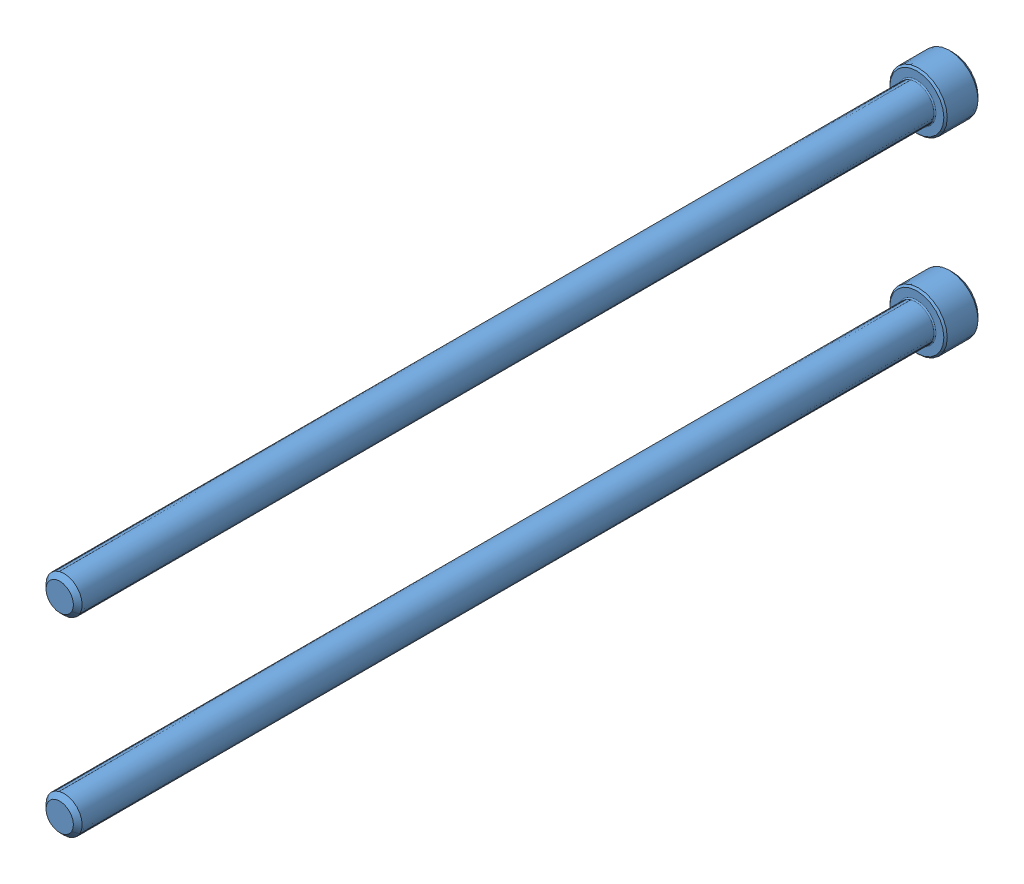
SolidWorks assembly WCP - GreyT Elevator (Cascade, 2 Stage) (1).step, configuration Default. Lengths in mm. (continued)
Components (placement in the parent): (continued)
- 10-32 SHCS - No Thread_WCP-0274 - 4.500.step-2: 10-32 SHCS - No Thread_WCP-0274 - 4.500.step [Default] at (165.1 1193.8 -77.7875) x (0.495006 -0.86889 0) z (0.86889 0.495006 0) size (7.67 119.13 7.67) (hidden)
- WCP-0326 Rev1.step-1: WCP-0326 Rev1.step [Default] at (165.1 1168.4 27.7749) x (0.127192 0.991878 0) z (0.991878 -0.127192 0) size (11.02 4.76 11) (hidden)
- WCP-0326 Rev1.step-2: WCP-0326 Rev1.step [Default] at (165.1 1193.8 27.7749) x (0.127192 0.991878 0) z (0.991878 -0.127192 0) size (11.02 4.76 11) (hidden)
- 10-32 BHCS - No Thread_WCP-0257 - 1.500.step-1: 10-32 BHCS - No Thread_WCP-0257 - 1.500.step [Default] at (101.6 1168.4 -101.6) x (-0.802481 0.596678 0) z (-0.596678 -0.802481 0) size (9.17 40.67 9.17) (hidden)
- 10-32 BHCS - No Thread_WCP-0257 - 1.500.step-2: 10-32 BHCS - No Thread_WCP-0257 - 1.500.step [Default] at (101.6 1193.8 -101.6) x (-0.802481 0.596678 0) z (-0.596678 -0.802481 0) size (9.17 40.67 9.17) (hidden)
- 10-32 BHCS - No Thread_WCP-0257 - 1.500.step-3: 10-32 BHCS - No Thread_WCP-0257 - 1.500.step [Default] at (76.2 1193.8 -101.6) x (-0.802481 0.596678 0) z (-0.596678 -0.802481 0) size (9.17 40.67 9.17) (hidden)
- 10-32 BHCS - No Thread_WCP-0257 - 1.500.step-4: 10-32 BHCS - No Thread_WCP-0257 - 1.500.step [Default] at (76.2 1168.4 -101.6) x (-0.802481 0.596678 0) z (-0.596678 -0.802481 0) size (9.17 40.67 9.17) (hidden)
- WCP-0326 Rev1.step-3: WCP-0326 Rev1.step [Default] at (101.6 1168.4 -67.4751) x (0.127192 0.991878 0) z (0.991878 -0.127192 0) size (11.02 4.76 11) (hidden)
- WCP-0326 Rev1.step-4: WCP-0326 Rev1.step [Default] at (101.6 1193.8 -67.4751) x (0.127192 0.991878 0) z (0.991878 -0.127192 0) size (11.02 4.76 11) (hidden)
- WCP-0326 Rev1.step-5: WCP-0326 Rev1.step [Default] at (76.2 1193.8 -67.4751) x (0.127192 0.991878 0) z (0.991878 -0.127192 0) size (11.02 4.76 11) (hidden)
- WCP-0326 Rev1.step-6: WCP-0326 Rev1.step [Default] at (76.2 1168.4 -67.4751) x (0.127192 0.991878 0) z (0.991878 -0.127192 0) size (11.02 4.76 11) (hidden)
- 10-32 BHCS - No Thread_WCP-0252 - 0.375.step-1: 10-32 BHCS - No Thread_WCP-0252 - 0.375.step [Default] at (165.1 11.1125 12.7) x (0.583861 0 0.811854) z (0.811854 0 -0.583861) size (9.17 12.1 9.17) (hidden)
- 10-32 BHCS - No Thread_WCP-0252 - 0.375.step-2: 10-32 BHCS - No Thread_WCP-0252 - 0.375.step [Default] at (165.1 11.1125 0) x (0.583861 0 0.811854) z (0.811854 0 -0.583861) size (9.17 12.1 9.17) (hidden)
- 10-32 BHCS - No Thread_WCP-0252 - 0.375.step-3: 10-32 BHCS - No Thread_WCP-0252 - 0.375.step [Default] at (165.1 11.1125 -12.7) x (0.583861 0 0.811854) z (0.811854 0 -0.583861) size (9.17 12.1 9.17) (hidden)
- 10-32 BHCS - No Thread_WCP-0252 - 0.375.step-4: 10-32 BHCS - No Thread_WCP-0252 - 0.375.step [Default] at (177.8 25.4 12.7) x (0 -0.948064 0.318079) z (0 0.318079 0.948064) size (9.17 12.1 9.17) (hidden)
- 10-32 BHCS - No Thread_WCP-0252 - 0.375.step-5: 10-32 BHCS - No Thread_WCP-0252 - 0.375.step [Default] at (177.8 25.4 0) x (0 -0.948064 0.318079) z (0 0.318079 0.948064) size (9.17 12.1 9.17) (hidden)
- 10-32 BHCS - No Thread_WCP-0252 - 0.375.step-6: 10-32 BHCS - No Thread_WCP-0252 - 0.375.step [Default] at (177.8 25.4 -12.7) x (0 -0.948064 0.318079) z (0 0.318079 0.948064) size (9.17 12.1 9.17) (hidden)
- 10-32 BHCS - No Thread_WCP-0252 - 0.375.step-7: 10-32 BHCS - No Thread_WCP-0252 - 0.375.step [Default] at (152.4 25.4 12.7) x (0 -0.983057 -0.183299) z (0 0.183299 -0.983057) size (9.17 12.1 9.17) (hidden)
- 10-32 BHCS - No Thread_WCP-0252 - 0.375.step-8: 10-32 BHCS - No Thread_WCP-0252 - 0.375.step [Default] at (152.4 25.4 0) x (0 -0.639879 0.768476) z (0 -0.768476 -0.639879) size (9.17 12.1 9.17) (hidden)
- 10-32 BHCS - No Thread_WCP-0252 - 0.375.step-9: 10-32 BHCS - No Thread_WCP-0252 - 0.375.step [Default] at (152.4 25.4 -12.7) x (0 -0.639879 0.768476) z (0 -0.768476 -0.639879) size (9.17 12.1 9.17) (hidden)
- 10-32 BHCS - No Thread_WCP-0252 - 0.375.step-10: 10-32 BHCS - No Thread_WCP-0252 - 0.375.step [Default] at (77.7875 50.8 -12.7) x (0 0.321661 0.946855) z (0 0.946855 -0.321661) size (9.17 12.1 9.17) (hidden)
- 10-32 BHCS - No Thread_WCP-0252 - 0.375.step-11: 10-32 BHCS - No Thread_WCP-0252 - 0.375.step [Default] at (77.7875 50.8 0) x (0 0.321661 0.946855) z (0 0.946855 -0.321661) size (9.17 12.1 9.17) (hidden)
- 10-32 BHCS - No Thread_WCP-0252 - 0.375.step-12: 10-32 BHCS - No Thread_WCP-0252 - 0.375.step [Default] at (77.7875 50.8 12.7) x (0 0.321661 0.946855) z (0 0.946855 -0.321661) size (9.17 12.1 9.17) (hidden)
- 10-32 BHCS - No Thread_WCP-0260 - 2.250.step-1: 10-32 BHCS - No Thread_WCP-0260 - 2.250.step [Default] at (76.2 1219.2 25.4) x (0.942963 -0.332897 0) z (-0.332897 -0.942963 0) size (9.17 59.72 9.17) (hidden)
- 10-32 BHCS - No Thread_WCP-0260 - 2.250.step-2: 10-32 BHCS - No Thread_WCP-0260 - 2.250.step [Default] at (101.6 1219.2 25.4) x (0.942963 -0.332897 0) z (-0.332897 -0.942963 0) size (9.17 59.72 9.17) (hidden)
- 10-32 BHCS - No Thread_WCP-0260 - 2.250.step-3: 10-32 BHCS - No Thread_WCP-0260 - 2.250.step [Default] at (76.2 25.4 25.4) x (0.942963 -0.332897 0) z (-0.332897 -0.942963 0) size (9.17 59.72 9.17) (hidden)
- 10-32 BHCS - No Thread_WCP-0260 - 2.250.step-4: 10-32 BHCS - No Thread_WCP-0260 - 2.250.step [Default] at (101.6 25.4 25.4) x (0.942963 -0.332897 0) z (-0.332897 -0.942963 0) size (9.17 59.72 9.17) (hidden)
- 10-32 BHCS - No Thread_WCP-0252 - 0.375.step-13: 10-32 BHCS - No Thread_WCP-0252 - 0.375.step [Default] at (63.5 50.8 25.4) x (0.796713 -0.604358 0) z (-0.604358 -0.796713 0) size (9.17 12.1 9.17) (hidden)
- 10-32 BHCS - No Thread_WCP-0252 - 0.375.step-14: 10-32 BHCS - No Thread_WCP-0252 - 0.375.step [Default] at (63.5 50.8 -25.4) x (-0.5764 -0.817168 0) z (0.817168 -0.5764 0) size (9.17 12.1 9.17) (hidden)
- 10-32 BHCS - No Thread_WCP-0252 - 0.375.step-15: 10-32 BHCS - No Thread_WCP-0252 - 0.375.step [Default] at (63.5 254 -25.4) x (-0.5764 -0.817168 0) z (0.817168 -0.5764 0) size (9.17 12.1 9.17) (hidden)
- 10-32 BHCS - No Thread_WCP-0252 - 0.375.step-16: 10-32 BHCS - No Thread_WCP-0252 - 0.375.step [Default] at (63.5 254 25.4) x (0.796713 -0.604358 0) z (-0.604358 -0.796713 0) size (9.17 12.1 9.17) (hidden)
- 10-32 BHCS - No Thread_WCP-0252 - 0.375.step-17: 10-32 BHCS - No Thread_WCP-0252 - 0.375.step [Default] at (77.7875 254 12.7) x (0 0.321661 0.946855) z (0 0.946855 -0.321661) size (9.17 12.1 9.17) (hidden)
- 10-32 BHCS - No Thread_WCP-0252 - 0.375.step-18: 10-32 BHCS - No Thread_WCP-0252 - 0.375.step [Default] at (77.7875 254 0) x (0 0.321661 0.946855) z (0 0.946855 -0.321661) size (9.17 12.1 9.17) (hidden)
- 10-32 BHCS - No Thread_WCP-0252 - 0.375.step-19: 10-32 BHCS - No Thread_WCP-0252 - 0.375.step [Default] at (77.7875 254 -12.7) x (0 0.321661 0.946855) z (0 0.946855 -0.321661) size (9.17 12.1 9.17) (hidden)
- 10-32 BHCS - No Thread_WCP-0252 - 0.375.step-20: 10-32 BHCS - No Thread_WCP-0252 - 0.375.step [Default] at (115.8875 1219.2 12.7) x (0 0.321661 0.946855) z (0 0.946855 -0.321661) size (9.17 12.1 9.17) (hidden)
- 10-32 BHCS - No Thread_WCP-0252 - 0.375.step-21: 10-32 BHCS - No Thread_WCP-0252 - 0.375.step [Default] at (115.8875 1219.2 0) x (0 0.321661 0.946855) z (0 0.946855 -0.321661) size (9.17 12.1 9.17) (hidden)
- 10-32 BHCS - No Thread_WCP-0252 - 0.375.step-22: 10-32 BHCS - No Thread_WCP-0252 - 0.375.step [Default] at (115.8875 1219.2 -12.7) x (0 0.321661 0.946855) z (0 0.946855 -0.321661) size (9.17 12.1 9.17) (hidden)
- 10-32 BHCS - No Thread_WCP-0252 - 0.375.step-23: 10-32 BHCS - No Thread_WCP-0252 - 0.375.step [Default] at (115.8875 25.4 -12.7) x (0 0.321661 0.946855) z (0 0.946855 -0.321661) size (9.17 12.1 9.17) (hidden)
- 10-32 BHCS - No Thread_WCP-0252 - 0.375.step-24: 10-32 BHCS - No Thread_WCP-0252 - 0.375.step [Default] at (115.8875 25.4 12.7) x (0 0.321661 0.946855) z (0 0.946855 -0.321661) size (9.17 12.1 9.17) (hidden)
- 10-32 BHCS - No Thread_WCP-0252 - 0.375.step-25: 10-32 BHCS - No Thread_WCP-0252 - 0.375.step [Default] at (115.8875 25.4 0) x (0 0.321661 0.946855) z (0 0.946855 -0.321661) size (9.17 12.1 9.17) (hidden)
- 10-32 BHCS - No Thread_WCP-0261 - 2.500.step-9: 10-32 BHCS - No Thread_WCP-0261 - 2.500.step [Default] at (38.1 25.4 25.4) x (-0.574084 -0.818796 0) z (-0.818796 0.574084 0) size (9.17 66.07 9.17) (hidden)
- 10-32 BHCS - No Thread_WCP-0261 - 2.500.step-10: 10-32 BHCS - No Thread_WCP-0261 - 2.500.step [Default] at (-50.8 25.4 25.4) x (-0.742698 -0.669626 0) z (-0.669626 0.742698 0) size (9.17 66.07 9.17) (hidden)
- 10-32 BHCS - No Thread_WCP-0261 - 2.500.step-11: 10-32 BHCS - No Thread_WCP-0261 - 2.500.step [Default] at (-38.1 25.4 25.4) x (-0.574084 -0.818796 0) z (-0.818796 0.574084 0) size (9.17 66.07 9.17) (hidden)
- 10-32 BHCS - No Thread_WCP-0261 - 2.500.step-12: 10-32 BHCS - No Thread_WCP-0261 - 2.500.step [Default] at (-25.4 25.4 25.4) x (-0.677804 -0.735243 0) z (-0.735243 0.677804 0) size (9.17 66.07 9.17) (hidden)
- WCP-0326 Rev1.step-7: WCP-0326 Rev1.step [Default] at (38.1 25.4 -31.7749) x (-0.281999 0.959415 0) z (-0.959415 -0.281999 0) size (11.02 4.76 11) (hidden)
- WCP-0326 Rev1.step-8: WCP-0326 Rev1.step [Default] at (12.7 25.4 -31.7749) x (-0.281999 0.959415 0) z (-0.959415 -0.281999 0) size (11.02 4.76 11) (hidden)
- WCP-0326 Rev1.step-9: WCP-0326 Rev1.step [Default] at (-25.4 25.4 -31.7749) x (-0.281999 0.959415 0) z (-0.959415 -0.281999 0) size (11.02 4.76 11) (hidden)
- WCP-0326 Rev1.step-10: WCP-0326 Rev1.step [Default] at (-38.1 25.4 -31.7749) x (-0.281999 0.959415 0) z (-0.959415 -0.281999 0) size (11.02 4.76 11) (hidden)
- WCP-0326 Rev1.step-11: WCP-0326 Rev1.step [Default] at (-50.8 25.4 -31.7749) x (-0.281999 0.959415 0) z (-0.959415 -0.281999 0) size (11.02 4.76 11) (hidden)
- WCP-0326 Rev1.step-12: WCP-0326 Rev1.step [Default] at (25.4 25.4 -31.7749) x (-0.281999 0.959415 0) z (-0.959415 -0.281999 0) size (11.02 4.76 11) (hidden)
- 10-32 BHCS - No Thread_WCP-0253 - 0.500.step-1: 10-32 BHCS - No Thread_WCP-0253 - 0.500.step [Default] at (-38.1 -25.4 23.114) x (0.542223 -0.840234 0) z (0.840234 0.542223 0) size (9.17 15.27 9.17) (hidden)
- 10-32 BHCS - No Thread_WCP-0253 - 0.500.step-2: 10-32 BHCS - No Thread_WCP-0253 - 0.500.step [Default] at (-12.7 -25.4 23.114) x (0.823635 -0.56712 0) z (0.56712 0.823635 0) size (9.17 15.27 9.17) (hidden)
- 10-32 BHCS - No Thread_WCP-0252 - 0.375.step-26: 10-32 BHCS - No Thread_WCP-0252 - 0.375.step [Default] at (-12.7 -11.1125 12.7) x (0.458328 0 0.888783) z (-0.888783 0 0.458328) size (9.17 12.1 9.17) (hidden)
- 10-32 BHCS - No Thread_WCP-0252 - 0.375.step-27: 10-32 BHCS - No Thread_WCP-0252 - 0.375.step [Default] at (-38.1 -11.1125 12.7) x (0.458328 0 0.888783) z (-0.888783 0 0.458328) size (9.17 12.1 9.17) (hidden)
- WCP-0326 Rev1.step-13: WCP-0326 Rev1.step [Default] at (-12.7 -17.3609 12.7) x (-0.884394 0 -0.466741) z (-0.466741 0 0.884394) size (11.02 4.76 11) (hidden)
- WCP-0326 Rev1.step-14: WCP-0326 Rev1.step [Default] at (-38.1 -17.3609 12.7) x (-0.806355 0 -0.591432) z (-0.591432 0 0.806355) size (11.02 4.76 11) (hidden)
- 10-32 BHCS - No Thread_WCP-0252 - 0.375.step-28: 10-32 BHCS - No Thread_WCP-0252 - 0.375.step [Default] at (165.1 25.4 25.4) x (0.238233 -0.971208 0) z (-0.971208 -0.238233 0) size (9.17 12.1 9.17) (hidden)
- 10-32 BHCS - No Thread_WCP-0252 - 0.375.step-29: 10-32 BHCS - No Thread_WCP-0252 - 0.375.step [Default] at (165.1 25.4 -25.4) x (0.705419 -0.708791 0) z (0.708791 0.705419 0) size (9.17 12.1 9.17) (hidden)
- #4-40 x .750L SHCS.step-1: #4-40 x .750L SHCS.step [Default] at (-4.1026 57.15 -50.8) x (0 0.222099 -0.975024) z (1 0 0) size (4.65 4.65 21.9) (hidden)
- NFS-0016_#4-40_thin_locknut_Default_As Machined_.step-1: NFS-0016_#4-40_thin_locknut_Default_As Machined_.step [Default] at (-10.35 57.15 -50.8) x (0 0.495484 -0.868617) z (0 0.868617 0.495484) size (6.37 2.79 7.35) (hidden)
- #4-40 x .750L SHCS.step-2: #4-40 x .750L SHCS.step [Default] at (-4.1026 31.75 -50.8) x (0 0.423366 0.905959) z (1 0 0) size (4.65 4.65 21.9) (hidden)
- #4-40 x .750L SHCS.step-3: #4-40 x .750L SHCS.step [Default] at (-4.1026 44.45 -50.8) x (0 -0.973772 0.227524) z (1 0 0) size (4.65 4.65 21.9) (hidden)
- NFS-0016_#4-40_thin_locknut_Default_As Machined_.step-2: NFS-0016_#4-40_thin_locknut_Default_As Machined_.step [Default] at (-10.35 44.45 -50.8) x (0 -0.910503 -0.413502) z (0 0.413502 -0.910503) size (6.37 2.79 7.35) (hidden)
- NFS-0016_#4-40_thin_locknut_Default_As Machined_.step-3: NFS-0016_#4-40_thin_locknut_Default_As Machined_.step [Default] at (-10.35 31.75 -50.8) x (0 0.495484 -0.868617) z (0 0.868617 0.495484) size (6.37 2.79 7.35) (hidden)
- 10-32 BHCS - No Thread_WCP-0261 - 2.500.step-13: 10-32 BHCS - No Thread_WCP-0261 - 2.500.step [Default] at (25.4 25.4 25.4) x (-0.992821 -0.119607 0) z (-0.119607 0.992821 0) size (9.17 66.07 9.17) (hidden)
- 10-32 BHCS - No Thread_WCP-0261 - 2.500.step-14: 10-32 BHCS - No Thread_WCP-0261 - 2.500.step [Default] at (12.7 25.4 25.4) x (-0.574084 -0.818796 0) z (-0.818796 0.574084 0) size (9.17 66.07 9.17) (hidden)
- 10-32 BHCS - No Thread_WCP-0263 - 3.000.step-1: 10-32 BHCS - No Thread_WCP-0263 - 3.000.step [Default] at (0 0 -38.1) x (0.756715 -0.653745 0) z (0.653745 0.756715 0) size (9.17 78.77 9.17) (hidden)
- 10-32 BHCS - No Thread_WCP-0263 - 3.000.step-2: 10-32 BHCS - No Thread_WCP-0263 - 3.000.step [Default] at (-50.8 0 -38.1) x (0.756715 -0.653745 0) z (0.653745 0.756715 0) size (9.17 78.77 9.17) (hidden)
- WCP-0571 Rev1.step-1: WCP-0571 Rev1.step [Default] at (-25.4 1181.1 -43.0403) size (15.88 15.88 15.71) (hidden)
- WCP-0571 Rev1.step-2: WCP-0571 Rev1.step [Default] at (-25.4 1181.1 -112.5347) x (-0.990411 -0.138152 0) z (0 0 -1) size (15.88 15.88 15.71) (hidden)
- 10-32 BHCS - No Thread_WCP-0257 - 1.500.step-5: 10-32 BHCS - No Thread_WCP-0257 - 1.500.step [Default] at (0 1181.1 -107.95) x (-0.802481 0.596678 0) z (-0.596678 -0.802481 0) size (9.17 40.67 9.17) (hidden)
- 10-32 BHCS - No Thread_WCP-0257 - 1.500.step-6: 10-32 BHCS - No Thread_WCP-0257 - 1.500.step [Default] at (-50.8 1181.1 -107.95) x (-0.853188 0.521603 0) z (-0.521603 -0.853188 0) size (9.17 40.67 9.17) (hidden)
- WCP-0560 Rev1.step-1: WCP-0560 Rev1.step [Default] at (-25.4 0 -50.8) x (-0.531612 0.846988 0) z (0 0 -1) size (47.96 47.68 9.53) (hidden)
- WCP-0560 Rev1.step-2: WCP-0560 Rev1.step [Default] at (-25.4 1181.1 -50.8) x (-0.820978 -0.57096 0) z (0 0 -1) size (47.96 47.68 9.53) (hidden)
- WCP-0583-023 Rev1.step-1: WCP-0583-023 Rev1.step [Default] at (-25.4 590.55 -50.8) x (-1 0 0) z (0 0 -1) size (50.36 1231.46 9) (hidden)
- 10-32 BHCS - No Thread_WCP-0261 - 2.500.step-15: 10-32 BHCS - No Thread_WCP-0261 - 2.500.step [Default] at (-165.1 1155.7 -30.1625) x (0.802481 0.596678 0) z (-0.596678 0.802481 0) size (9.17 66.07 9.17) (hidden)
- 10-32 BHCS - No Thread_WCP-0261 - 2.500.step-16: 10-32 BHCS - No Thread_WCP-0261 - 2.500.step [Default] at (-165.1 1143 30.1625) x (-0.999937 0.011255 0) z (0.011255 0.999937 0) size (9.17 66.07 9.17) (hidden)
- WCP-EX-0019-008.step-1: WCP-EX-0019-008.step [Default] at (88.9 31.75 -50.8) size (3 1228.38 34.58) (hidden)
- WCP-0583-015 Rev1.step-1: WCP-0583-015 Rev1.step [Default] at (88.9 1181.1 -73.025) size (34.92 38.1 6.35) (hidden)
- WCP-0476 Rev1.step-1: WCP-0476 Rev1.step [Default] at (-25.4 0 -34.925) size (63.5 34.92 6.35) (hidden)
- WCP-0476 Rev1.step-2: WCP-0476 Rev1.step [Default] at (-25.4 1181.1 -73.025) size (63.5 34.92 6.35) (hidden)
- WCP-0476 Rev1.step-3: WCP-0476 Rev1.step [Default] at (-25.4 1181.1 -104.775) size (63.5 34.92 6.35) (hidden)
- WCP-0583-025 Rev1_DefaultSM-FLAT-PATTERN.step-1: WCP-0583-025 Rev1_DefaultSM-FLAT-PATTERN.step [Default] at (22.225 25.4 -29.4) x (-1 0 0) z (0 0 -1) size (44.45 50.8 31.75) (hidden)
- WCP-0583-026 Rev1.step-1: WCP-0583-026 Rev1.step [Default] at (-31.75 25.4 -29.4) x (-1 0 0) z (0 0 -1) size (50.8 50.8 31.75) (hidden)
- WCP-0207 Rev1.step-1: WCP-0207 Rev1.step [Default] at (165.1 1193.8 -50.8) x (0 0 -1) z (0.999873 -0.015939 0) size (50.8 9.5 9.5) (hidden)
- WCP-0207 Rev1.step-2: WCP-0207 Rev1.step [Default] at (165.1 1168.4 -50.8) x (0 0 -1) z (0.999873 -0.015939 0) size (50.8 9.5 9.5) (hidden)
- WCP-0308 Rev1.step-1: WCP-0308 Rev1.step [Default] at (-50.8 0 -28.575) x (0 0 -1) z (0.995626 0.093431 0) size (6.35 9.5 9.5) (hidden)
- WCP-0308 Rev1.step-2: WCP-0308 Rev1.step [Default] at (0 0 -28.575) x (0 0 -1) z (0.995626 0.093431 0) size (6.35 9.5 9.5) (hidden)
- WCP-0307 Rev1.step-1: WCP-0307 Rev1.step [Default] at (-12.7 -25.4 26.9913) x (0 0 1) z (-0.952187 0.305516 0) size (3.18 9.5 9.5) (hidden)
- WCP-0307 Rev1.step-2: WCP-0307 Rev1.step [Default] at (-38.1 -25.4 26.9913) x (0 0 1) z (-0.952187 0.305516 0) size (3.18 9.5 9.5) (hidden)
- WCP-0307 Rev1.step-3: WCP-0307 Rev1.step [Default] at (0 0 26.9913) x (0 0 1) z (-0.952187 0.305516 0) size (3.18 9.5 9.5) (hidden)
- WCP-0307 Rev1.step-4: WCP-0307 Rev1.step [Default] at (-50.8 0 26.9913) x (0 0 1) z (-0.952187 0.305516 0) size (3.18 9.5 9.5) (hidden)
- WCP-0599 Rev1.step-1: WCP-0599 Rev1.step [Default] at (-25.4 1181.1 -77.7875) x (0 0 -1) z (0.982361 -0.186992 0) size (63.5 12.67 13.72) (hidden)
- WCP-0790_500L_500_hex.step-1: WCP-0790_500L_500_hex.step [Default] at (-25.4 1181.1 -61.9125) x (0.991671 -0.128795 0) z (0 0 1) size (19.5 19.5 12.7) (hidden)
- WCP-0789_250L_500_hex.step-1: WCP-0789_250L_500_hex.step [Default] at (-25.4 0 -42.8625) size (19.5 19.5 6.35) (hidden)
- 10-32 BHCS - No Thread_WCP-0261 - 2.500.step-17: 10-32 BHCS - No Thread_WCP-0261 - 2.500.step [Default] at (-127 63.5 30.1625) x (-0.985295 -0.170861 0) z (-0.170861 0.985295 0) size (9.17 66.07 9.17) (hidden)
- 10-32 BHCS - No Thread_WCP-0261 - 2.500.step-18: 10-32 BHCS - No Thread_WCP-0261 - 2.500.step [Default] at (-127 50.8 -30.1625) x (0.742242 0.670132 0) z (-0.670132 0.742242 0) size (9.17 66.07 9.17) (hidden)
- WCP-0374 Rev1.step-1: WCP-0374 Rev1.step [Default] at (165.1 22.225 0) x (0 0 -1) z (1 0 0) size (44.07 19.05 18.67) (hidden)
- WCP-0379 Rev1.step-1: WCP-0379 Rev1.step [Default] at (165.1 22.225 0) x (0 0 -1) z (1 0 0) size (47.24 20.64 21.84) (hidden)
- WCP-0379 Rev1.step-2: WCP-0379 Rev1.step [Default] at (66.675 50.8 0) x (0 0 -1) z (0 1 0) size (47.24 20.64 21.84) (hidden)
- WCP-0374 Rev1.step-2: WCP-0374 Rev1.step [Default] at (66.675 50.8 0) x (0 0 -1) z (0 1 0) size (44.07 19.05 18.67) (hidden)
- WCP-0374 Rev1.step-3: WCP-0374 Rev1.step [Default] at (66.675 254 0) x (0 0 -1) z (0 1 0) size (44.07 19.05 18.67) (hidden)
- WCP-0379 Rev1.step-3: WCP-0379 Rev1.step [Default] at (66.675 254 0) x (0 0 -1) z (0 1 0) size (47.24 20.64 21.84) (hidden)
- WCP-0374 Rev1.step-4: WCP-0374 Rev1.step [Default] at (104.775 1219.2 0) x (0 0 -1) z (0 1 0) size (44.07 19.05 18.67) (hidden)
- WCP-0379 Rev1.step-4: WCP-0379 Rev1.step [Default] at (104.775 1219.2 0) x (0 0 -1) z (0 1 0) size (47.24 20.64 21.84) (hidden)
- WCP-0379 Rev1.step-5: WCP-0379 Rev1.step [Default] at (104.775 25.4 0) x (0 0 -1) z (0 1 0) size (47.24 20.64 21.84) (hidden)
- WCP-0374 Rev1.step-5: WCP-0374 Rev1.step [Default] at (104.775 25.4 0) x (0 0 -1) z (0 1 0) size (44.07 19.05 18.67) (hidden)
- WCP-0785_0_500_flanged_thunderhex_bearing.step-1: WCP-0785_0_500_flanged_thunderhex_bearing.step [Default] at (-25.4 0 -35.7188) x (-0.952019 0.30604 0) z (0 0 -1) size (31.12 31.12 7.94) (hidden)
- WCP-0785_0_500_flanged_thunderhex_bearing.step-2: WCP-0785_0_500_flanged_thunderhex_bearing.step [Default] at (-25.4 1181.1 -105.5688) x (-0.914179 0.405311 0) z (0 0 -1) size (31.12 31.12 7.94) (hidden)
- WCP-0785_0_500_flanged_thunderhex_bearing.step-3: WCP-0785_0_500_flanged_thunderhex_bearing.step [Default] at (-25.4 1181.1 -72.2313) x (0.656952 0.753932 0) z (0 0 1) size (31.12 31.12 7.94) (hidden)
- WCP-0800_500_hex_collar_high_strength.step-1: WCP-0800_500_hex_collar_high_strength.step [Default] at (-25.4 0 -60.325) size (28.56 28.57 9.53) (hidden)
- 10-32 BHCS - No Thread_WCP-0261 - 2.500.step-19: 10-32 BHCS - No Thread_WCP-0261 - 2.500.step [Default] at (-88.9 76.2 -30.1625) x (0.742242 0.670132 0) z (-0.670132 0.742242 0) size (9.17 66.07 9.17) (hidden)
- 10-32 BHCS - No Thread_WCP-0261 - 2.500.step-20: 10-32 BHCS - No Thread_WCP-0261 - 2.500.step [Default] at (-88.9 88.9 30.1625) x (-0.985295 -0.170861 0) z (-0.170861 0.985295 0) size (9.17 66.07 9.17) (hidden)
- 10-32 BHCS - No Thread_WCP-0261 - 2.500.step-21: 10-32 BHCS - No Thread_WCP-0261 - 2.500.step [Default] at (-88.9 228.6 30.1625) x (-0.985295 -0.170861 0) z (-0.170861 0.985295 0) size (9.17 66.07 9.17) (hidden)
- 10-32 BHCS - No Thread_WCP-0261 - 2.500.step-22: 10-32 BHCS - No Thread_WCP-0261 - 2.500.step [Default] at (-88.9 215.9 -30.1625) x (0.742242 0.670132 0) z (-0.670132 0.742242 0) size (9.17 66.07 9.17) (hidden)
- WCP-EX-0019-008.step-2: WCP-EX-0019-008.step [Default] at (-88.9 31.75 -50.8) size (3 1228.38 34.58) (hidden)
- WCP-0583-015 Rev1.step-2: WCP-0583-015 Rev1.step [Default] at (-88.9 1181.1 -73.025) x (-1 0 0) z (0 0 -1) size (34.92 38.1 6.35) (hidden)
- WCP-0326 Rev1.step-15: WCP-0326 Rev1.step [Default] at (-165.1 1193.8 27.7749) x (-0.127192 0.991878 0) z (0.991878 0.127192 0) size (11.02 4.76 11) (hidden)
- 10-32 SHCS - No Thread_WCP-0274 - 4.500.step-3: 10-32 SHCS - No Thread_WCP-0274 - 4.500.step [Default] at (-165.1 1193.8 -77.7875) x (-0.495006 -0.86889 0) z (0.86889 -0.495006 0) size (7.67 119.13 7.67)
- WCP-0326 Rev1.step-16: WCP-0326 Rev1.step [Default] at (-165.1 1168.4 27.7749) x (-0.127192 0.991878 0) z (0.991878 0.127192 0) size (11.02 4.76 11) (hidden)
- 10-32 SHCS - No Thread_WCP-0274 - 4.500.step-4: 10-32 SHCS - No Thread_WCP-0274 - 4.500.step [Default] at (-165.1 1168.4 -77.7875) x (-0.495006 -0.86889 0) z (0.86889 -0.495006 0) size (7.67 119.13 7.67)
- 10-32 BHCS - No Thread_WCP-0257 - 1.500.step-7: 10-32 BHCS - No Thread_WCP-0257 - 1.500.step [Default] at (-101.6 1193.8 -101.6) x (0.802481 0.596678 0) z (-0.596678 0.802481 0) size (9.17 40.67 9.17) (hidden)
- WCP-0326 Rev1.step-17: WCP-0326 Rev1.step [Default] at (-101.6 1193.8 -67.4751) x (-0.127192 0.991878 0) z (0.991878 0.127192 0) size (11.02 4.76 11) (hidden)
- 10-32 BHCS - No Thread_WCP-0257 - 1.500.step-8: 10-32 BHCS - No Thread_WCP-0257 - 1.500.step [Default] at (-101.6 1168.4 -101.6) x (0.802481 0.596678 0) z (-0.596678 0.802481 0) size (9.17 40.67 9.17) (hidden)
- WCP-0326 Rev1.step-18: WCP-0326 Rev1.step [Default] at (-101.6 1168.4 -67.4751) x (-0.127192 0.991878 0) z (0.991878 0.127192 0) size (11.02 4.76 11) (hidden)
- WCP-0326 Rev1.step-19: WCP-0326 Rev1.step [Default] at (-76.2 1168.4 -67.4751) x (-0.127192 0.991878 0) z (0.991878 0.127192 0) size (11.02 4.76 11) (hidden)
- 10-32 BHCS - No Thread_WCP-0257 - 1.500.step-9: 10-32 BHCS - No Thread_WCP-0257 - 1.500.step [Default] at (-76.2 1168.4 -101.6) x (0.802481 0.596678 0) z (-0.596678 0.802481 0) size (9.17 40.67 9.17) (hidden)
- 10-32 BHCS - No Thread_WCP-0257 - 1.500.step-10: 10-32 BHCS - No Thread_WCP-0257 - 1.500.step [Default] at (-76.2 1193.8 -101.6) x (0.802481 0.596678 0) z (-0.596678 0.802481 0) size (9.17 40.67 9.17) (hidden)
- WCP-0326 Rev1.step-20: WCP-0326 Rev1.step [Default] at (-76.2 1193.8 -67.4751) x (-0.127192 0.991878 0) z (0.991878 0.127192 0) size (11.02 4.76 11) (hidden)
- 10-32 BHCS - No Thread_WCP-0260 - 2.250.step-5: 10-32 BHCS - No Thread_WCP-0260 - 2.250.step [Default] at (-101.6 25.4 25.4) x (-0.942963 -0.332897 0) z (-0.332897 0.942963 0) size (9.17 59.72 9.17) (hidden)
- 10-32 BHCS - No Thread_WCP-0260 - 2.250.step-6: 10-32 BHCS - No Thread_WCP-0260 - 2.250.step [Default] at (-76.2 25.4 25.4) x (-0.942963 -0.332897 0) z (-0.332897 0.942963 0) size (9.17 59.72 9.17) (hidden)
- 10-32 BHCS - No Thread_WCP-0252 - 0.375.step-30: 10-32 BHCS - No Thread_WCP-0252 - 0.375.step [Default] at (-63.5 50.8 25.4) x (-0.796713 -0.604358 0) z (-0.604358 0.796713 0) size (9.17 12.1 9.17) (hidden)
- WCP-0379 Rev1.step-6: WCP-0379 Rev1.step [Default] at (-104.775 25.4 0) x (0 0 -1) z (0 -1 0) size (47.24 20.64 21.84) (hidden)
- WCP-0374 Rev1.step-6: WCP-0374 Rev1.step [Default] at (-104.775 25.4 0) x (0 0 -1) z (0 -1 0) size (44.07 19.05 18.67) (hidden)
- 10-32 BHCS - No Thread_WCP-0252 - 0.375.step-31: 10-32 BHCS - No Thread_WCP-0252 - 0.375.step [Default] at (-115.8875 25.4 0) x (0 0.321661 0.946855) z (0 -0.946855 0.321661) size (9.17 12.1 9.17) (hidden)
- 10-32 BHCS - No Thread_WCP-0252 - 0.375.step-32: 10-32 BHCS - No Thread_WCP-0252 - 0.375.step [Default] at (-115.8875 25.4 -12.7) x (0 0.321661 0.946855) z (0 -0.946855 0.321661) size (9.17 12.1 9.17) (hidden)
- 10-32 BHCS - No Thread_WCP-0252 - 0.375.step-33: 10-32 BHCS - No Thread_WCP-0252 - 0.375.step [Default] at (-115.8875 25.4 12.7) x (0 0.321661 0.946855) z (0 -0.946855 0.321661) size (9.17 12.1 9.17) (hidden)
- 10-32 BHCS - No Thread_WCP-0252 - 0.375.step-34: 10-32 BHCS - No Thread_WCP-0252 - 0.375.step [Default] at (-77.7875 50.8 0) x (0 0.321661 0.946855) z (0 -0.946855 0.321661) size (9.17 12.1 9.17) (hidden)
- 10-32 BHCS - No Thread_WCP-0252 - 0.375.step-35: 10-32 BHCS - No Thread_WCP-0252 - 0.375.step [Default] at (-77.7875 50.8 12.7) x (0 0.321661 0.946855) z (0 -0.946855 0.321661) size (9.17 12.1 9.17) (hidden)
- 10-32 BHCS - No Thread_WCP-0252 - 0.375.step-36: 10-32 BHCS - No Thread_WCP-0252 - 0.375.step [Default] at (-77.7875 50.8 -12.7) x (0 0.321661 0.946855) z (0 -0.946855 0.321661) size (9.17 12.1 9.17) (hidden)
- 10-32 BHCS - No Thread_WCP-0252 - 0.375.step-37: 10-32 BHCS - No Thread_WCP-0252 - 0.375.step [Default] at (-63.5 50.8 -25.4) x (0.5764 -0.817168 0) z (0.817168 0.5764 0) size (9.17 12.1 9.17) (hidden)
- 10-32 BHCS - No Thread_WCP-0252 - 0.375.step-38: 10-32 BHCS - No Thread_WCP-0252 - 0.375.step [Default] at (-177.8 25.4 12.7) x (0 -0.948064 0.318079) z (0 -0.318079 -0.948064) size (9.17 12.1 9.17) (hidden)
- 10-32 BHCS - No Thread_WCP-0252 - 0.375.step-39: 10-32 BHCS - No Thread_WCP-0252 - 0.375.step [Default] at (-177.8 25.4 0) x (0 -0.948064 0.318079) z (0 -0.318079 -0.948064) size (9.17 12.1 9.17) (hidden)
- 10-32 BHCS - No Thread_WCP-0252 - 0.375.step-40: 10-32 BHCS - No Thread_WCP-0252 - 0.375.step [Default] at (-177.8 25.4 -12.7) x (0 -0.948064 0.318079) z (0 -0.318079 -0.948064) size (9.17 12.1 9.17) (hidden)
- 10-32 BHCS - No Thread_WCP-0252 - 0.375.step-41: 10-32 BHCS - No Thread_WCP-0252 - 0.375.step [Default] at (-152.4 25.4 12.7) x (0 -0.983057 -0.183299) z (0 -0.183299 0.983057) size (9.17 12.1 9.17) (hidden)
- 10-32 BHCS - No Thread_WCP-0252 - 0.375.step-42: 10-32 BHCS - No Thread_WCP-0252 - 0.375.step [Default] at (-152.4 25.4 0) x (0 -0.639879 0.768476) z (0 0.768476 0.639879) size (9.17 12.1 9.17) (hidden)
- 10-32 BHCS - No Thread_WCP-0252 - 0.375.step-43: 10-32 BHCS - No Thread_WCP-0252 - 0.375.step [Default] at (-152.4 25.4 -12.7) x (0 -0.639879 0.768476) z (0 0.768476 0.639879) size (9.17 12.1 9.17) (hidden)
- WCP-0379 Rev1.step-7: WCP-0379 Rev1.step [Default] at (-165.1 22.225 0) x (0 0 -1) z (1 0 0) size (47.24 20.64 21.84) (hidden)
- WCP-0374 Rev1.step-7: WCP-0374 Rev1.step [Default] at (-165.1 22.225 0) x (0 0 -1) z (1 0 0) size (44.07 19.05 18.67) (hidden)
- 10-32 BHCS - No Thread_WCP-0252 - 0.375.step-44: 10-32 BHCS - No Thread_WCP-0252 - 0.375.step [Default] at (-165.1 11.1125 -12.7) x (-0.583861 0 0.811854) z (0.811854 0 0.583861) size (9.17 12.1 9.17) (hidden)
- 10-32 BHCS - No Thread_WCP-0252 - 0.375.step-45: 10-32 BHCS - No Thread_WCP-0252 - 0.375.step [Default] at (-165.1 11.1125 0) x (-0.583861 0 0.811854) z (0.811854 0 0.583861) size (9.17 12.1 9.17) (hidden)
- 10-32 BHCS - No Thread_WCP-0252 - 0.375.step-46: 10-32 BHCS - No Thread_WCP-0252 - 0.375.step [Default] at (-165.1 11.1125 12.7) x (-0.583861 0 0.811854) z (0.811854 0 0.583861) size (9.17 12.1 9.17) (hidden)
- 10-32 BHCS - No Thread_WCP-0252 - 0.375.step-47: 10-32 BHCS - No Thread_WCP-0252 - 0.375.step [Default] at (-63.5 254 -25.4) x (0.5764 -0.817168 0) z (0.817168 0.5764 0) size (9.17 12.1 9.17) (hidden)
- WCP-0379 Rev1.step-8: WCP-0379 Rev1.step [Default] at (-66.675 254 0) x (0 0 -1) z (0 -1 0) size (47.24 20.64 21.84) (hidden)
- WCP-0374 Rev1.step-8: WCP-0374 Rev1.step [Default] at (-66.675 254 0) x (0 0 -1) z (0 -1 0) size (44.07 19.05 18.67) (hidden)
- 10-32 BHCS - No Thread_WCP-0252 - 0.375.step-48: 10-32 BHCS - No Thread_WCP-0252 - 0.375.step [Default] at (-77.7875 254 -12.7) x (0 0.321661 0.946855) z (0 -0.946855 0.321661) size (9.17 12.1 9.17) (hidden)
- 10-32 BHCS - No Thread_WCP-0252 - 0.375.step-49: 10-32 BHCS - No Thread_WCP-0252 - 0.375.step [Default] at (-77.7875 254 0) x (0 0.321661 0.946855) z (0 -0.946855 0.321661) size (9.17 12.1 9.17) (hidden)
- 10-32 BHCS - No Thread_WCP-0252 - 0.375.step-50: 10-32 BHCS - No Thread_WCP-0252 - 0.375.step [Default] at (-77.7875 254 12.7) x (0 0.321661 0.946855) z (0 -0.946855 0.321661) size (9.17 12.1 9.17) (hidden)
- 10-32 BHCS - No Thread_WCP-0252 - 0.375.step-51: 10-32 BHCS - No Thread_WCP-0252 - 0.375.step [Default] at (-63.5 254 25.4) x (-0.796713 -0.604358 0) z (-0.604358 0.796713 0) size (9.17 12.1 9.17) (hidden)
- 10-32 BHCS - No Thread_WCP-0260 - 2.250.step-7: 10-32 BHCS - No Thread_WCP-0260 - 2.250.step [Default] at (-101.6 1219.2 25.4) x (-0.942963 -0.332897 0) z (-0.332897 0.942963 0) size (9.17 59.72 9.17) (hidden)
- 10-32 BHCS - No Thread_WCP-0260 - 2.250.step-8: 10-32 BHCS - No Thread_WCP-0260 - 2.250.step [Default] at (-76.2 1219.2 25.4) x (-0.942963 -0.332897 0) z (-0.332897 0.942963 0) size (9.17 59.72 9.17) (hidden)
- 10-32 BHCS - No Thread_WCP-0252 - 0.375.step-52: 10-32 BHCS - No Thread_WCP-0252 - 0.375.step [Default] at (-115.8875 1219.2 12.7) x (0 0.321661 0.946855) z (0 -0.946855 0.321661) size (9.17 12.1 9.17) (hidden)
- 10-32 BHCS - No Thread_WCP-0252 - 0.375.step-53: 10-32 BHCS - No Thread_WCP-0252 - 0.375.step [Default] at (-115.8875 1219.2 0) x (0 0.321661 0.946855) z (0 -0.946855 0.321661) size (9.17 12.1 9.17) (hidden)
- 10-32 BHCS - No Thread_WCP-0252 - 0.375.step-54: 10-32 BHCS - No Thread_WCP-0252 - 0.375.step [Default] at (-115.8875 1219.2 -12.7) x (0 0.321661 0.946855) z (0 -0.946855 0.321661) size (9.17 12.1 9.17) (hidden)
- WCP-0379 Rev1.step-9: WCP-0379 Rev1.step [Default] at (-104.775 1219.2 0) x (0 0 -1) z (0 -1 0) size (47.24 20.64 21.84) (hidden)
- WCP-0374 Rev1.step-9: WCP-0374 Rev1.step [Default] at (-104.775 1219.2 0) x (0 0 -1) z (0 -1 0) size (44.07 19.05 18.67) (hidden)
- WCP-0379 Rev1.step-10: WCP-0379 Rev1.step [Default] at (-66.675 50.8 0) x (0 0 -1) z (0 -1 0) size (47.24 20.64 21.84) (hidden)
- WCP-0374 Rev1.step-10: WCP-0374 Rev1.step [Default] at (-66.675 50.8 0) x (0 0 -1) z (0 -1 0) size (44.07 19.05 18.67) (hidden)
- WCP-0207 Rev1.step-3: WCP-0207 Rev1.step [Default] at (-165.1 1193.8 -50.8) x (0 0 -1) z (0.999873 0.015939 0) size (50.8 9.5 9.5) (hidden)
- WCP-0207 Rev1.step-4: WCP-0207 Rev1.step [Default] at (-165.1 1168.4 -50.8) x (0 0 -1) z (0.999873 0.015939 0) size (50.8 9.5 9.5) (hidden)
- 10-32 BHCS - No Thread_WCP-0252 - 0.375.step-55: 10-32 BHCS - No Thread_WCP-0252 - 0.375.step [Default] at (-165.1 25.4 25.4) x (-0.238233 -0.971208 0) z (-0.971208 0.238233 0) size (9.17 12.1 9.17) (hidden)
- 10-32 BHCS - No Thread_WCP-0252 - 0.375.step-56: 10-32 BHCS - No Thread_WCP-0252 - 0.375.step [Default] at (-165.1 25.4 -25.4) x (-0.705419 -0.708791 0) z (0.708791 -0.705419 0) size (9.17 12.1 9.17) (hidden)
- WCP-EX-0019-004.step-2: WCP-EX-0019-004.step [Default] at (-127 622.3 0) x (0 1 0) z (1 0 0) size (1219.2 50.8 25.4) (hidden)
- MirrorWCP-EX-0019-005.step-1: MirrorWCP-EX-0019-005.step [Default] at (-88.9 152.4 0) x (0 -1 0) z (-1 0 0) size (228.6 50.8 25.4) (hidden)
- WCP-0523 Rev1.step-1: WCP-0523 Rev1.step [Default] at (88.9 152.4 -41.6719) x (0.995786 -0.091702 0) z (-0.091702 -0.995786 0) size (15.88 0.79 15.88) (hidden)
- 10-32 BHCS - No Thread_WCP-0263 - 3.000.step-3: 10-32 BHCS - No Thread_WCP-0263 - 3.000.step [Default] at (88.9 152.4 -42.0688) x (0.163054 -0.986617 0) z (0.986617 0.163054 0) size (9.17 78.77 9.17) (hidden)
- WCP-0326 Rev1.step-21: WCP-0326 Rev1.step [Default] at (88.9 152.4 27.7749) x (0.982047 -0.188635 0) z (-0.188635 -0.982047 0) size (11.02 4.76 11) (hidden)
- WCP-0523 Rev1.step-2: WCP-0523 Rev1.step [Default] at (-88.9 152.4 -41.6719) x (0.726757 0.686895 0) z (0.686895 -0.726757 0) size (15.88 0.79 15.88) (hidden)
- WCP-0326 Rev1.step-22: WCP-0326 Rev1.step [Default] at (-88.9 152.4 27.7749) x (0.925745 -0.378148 0) z (-0.378148 -0.925745 0) size (11.02 4.76 11) (hidden)
- 10-32 BHCS - No Thread_WCP-0263 - 3.000.step-4: 10-32 BHCS - No Thread_WCP-0263 - 3.000.step [Default] at (-88.9 152.4 -42.0688) x (0.163054 -0.986617 0) z (0.986617 0.163054 0) size (9.17 78.77 9.17) (hidden)
- WCP-0203 Rev1.step-1: WCP-0203 Rev1.step [Default] at (88.9 152.4 -33.3375) x (0 0 1) z (0.991701 -0.128564 0) size (15.88 9.5 9.5) (hidden)
- WCP-0203 Rev1.step-2: WCP-0203 Rev1.step [Default] at (-88.9 152.4 -33.3375) x (0 0 1) z (-0.976351 -0.216192 0) size (15.88 9.5 9.5) (hidden)
- WCP-0583-027 Rev1.step-1: WCP-0583-027 Rev1.step [Default] at (-38.1 -12.7 25.4) x (0 -1 0) z (1 0 0) size (25.4 25.4 50.8) (hidden)
